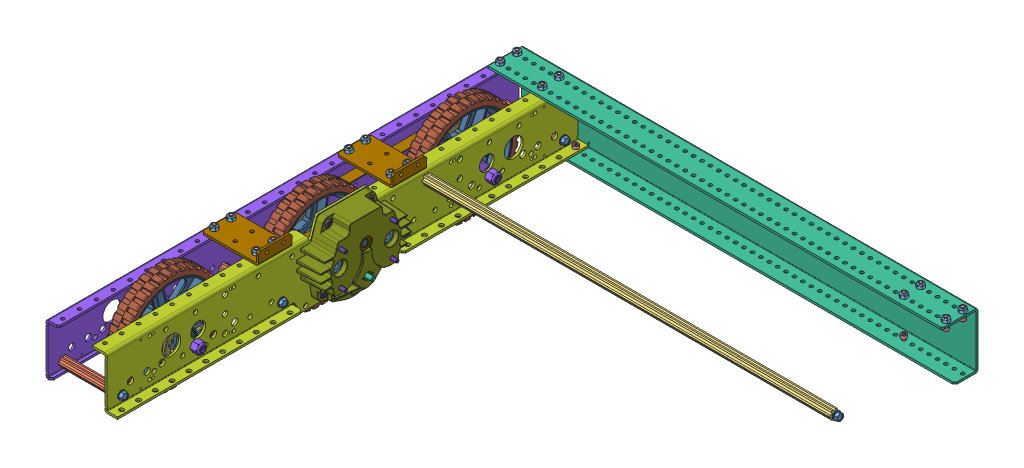
SolidWorks assembly AM14U3 Square Half, configuration Default. Lengths in mm.
Overall size (722.96 215.27 715.14).
150 component instances, 35 part files, 6 mates.
Components (placement in the parent):
- AM14U3 Square Frame Half-1: AM14U3 Square Frame Half [Default] at (326.068 37.2757 -291.2758) size (722.38 116.33 715.14)
  - ThreadRollingScrew_0.25-20x0.75_FHTS 0.25-20-G-0.75-C-1: ThreadRollingScrew_0.25-20x0.75_FHTS 0.25-20-G-0.75-C [Default] at (-600.075 -67.691 639.064) x (-1 0 0) z (0 0.924225 0.381849) size (24.64 12.19 12.19)
  - ThreadRollingScrew_0.25-20x0.75_FHTS 0.25-20-G-0.75-C-2: ThreadRollingScrew_0.25-20x0.75_FHTS 0.25-20-G-0.75-C [Default] at (-600.075 -67.691 -27.94) x (-1 0 0) z (0 0.924225 0.381849) size (24.64 12.19 12.19)
  - ThreadRollingScrew_0.25-20x0.75_FHTS 0.25-20-G-0.75-C-3: ThreadRollingScrew_0.25-20x0.75_FHTS 0.25-20-G-0.75-C [Default] at (-692.15 -67.691 -27.813) size (24.64 12.19 12.19)
  - ThreadRollingScrew_0.25-20x0.75_FHTS 0.25-20-G-0.75-C-4: ThreadRollingScrew_0.25-20x0.75_FHTS 0.25-20-G-0.75-C [Default] at (-603.25 -15.494 178.562) size (24.64 12.19 12.19)
  - ThreadRollingScrew_0.25-20x0.75_FHTS 0.25-20-G-0.75-C-5: ThreadRollingScrew_0.25-20x0.75_FHTS 0.25-20-G-0.75-C [Default] at (-692.15 -67.691 638.937) size (24.64 12.19 12.19)
  - ThreadRollingScrew_0.25-20x0.75_FHTS 0.25-20-G-0.75-C-6: ThreadRollingScrew_0.25-20x0.75_FHTS 0.25-20-G-0.75-C [Default] at (19.05 -15.494 178.562) x (-1 0 0) z (0 0.525103 -0.851039) size (24.64 12.19 12.19)
  - 500Churro_3.375-1: 500Churro_3.375 [Default] at (-603.25 -67.691 -27.813) x (0 -0.866025 0.5) z (-1 0 0) size (14.66 12.7 85.72)
  - 500Churro_3.375-2: 500Churro_3.375 [Default] at (-603.25 -67.691 638.937) x (0 -0.866025 0.5) z (-1 0 0) size (14.66 12.7 85.72)
  - 500Churro_24.25-1: 500Churro_24.25 [Default] at (15.875 -15.494 178.562) x (0 0 -1) z (-1 0 0) size (14.66 12.7 615.95)
  - Screw_SHCS_10-32x0.5_HX-SHCS 0.19-32x1.375x1-C-1: Screw_SHCS_10-32x0.5_HX-SHCS 0.19-32x1.375x1-C [Default] at (-679.45 -11.43 -11.938) x (0 1 0) z (-0.440454 0 0.897775) size (17.53 7.94 7.94)
  - Screw_SHCS_10-32x0.5_HX-SHCS 0.19-32x1.375x1-C-2: Screw_SHCS_10-32x0.5_HX-SHCS 0.19-32x1.375x1-C [Default] at (-679.45 -11.43 -37.338) x (0 1 0) z (-0.063425 0 0.997987) size (17.53 7.94 7.94)
  - Screw_SHCS_10-32x0.5_HX-SHCS 0.19-32x1.375x1-C-3: Screw_SHCS_10-32x0.5_HX-SHCS 0.19-32x1.375x1-C [Default] at (-615.95 -11.43 -37.338) x (0 1 0) z (0 0 1) size (17.53 7.94 7.94)
  - Screw_SHCS_10-32x0.5_HX-SHCS 0.19-32x1.375x1-C-4: Screw_SHCS_10-32x0.5_HX-SHCS 0.19-32x1.375x1-C [Default] at (-615.95 -11.43 -11.938) x (0 1 0) z (0 0 1) size (17.53 7.94 7.94)
  - Screw_SHCS_10-32x0.5_HX-SHCS 0.19-32x1.375x1-C-5: Screw_SHCS_10-32x0.5_HX-SHCS 0.19-32x1.375x1-C [Default] at (-590.55 -73.152 -37.338) x (0 -1 0) z (0 0 1) size (17.53 7.94 7.94)
  - Screw_SHCS_10-32x0.5_HX-SHCS 0.19-32x1.375x1-C-6: Screw_SHCS_10-32x0.5_HX-SHCS 0.19-32x1.375x1-C [Default] at (-6.35 -11.176 -37.338) x (0 1 0) z (0.222581 0 0.974914) size (17.53 7.94 7.94)
  - Screw_SHCS_10-32x0.5_HX-SHCS 0.19-32x1.375x1-C-7: Screw_SHCS_10-32x0.5_HX-SHCS 0.19-32x1.375x1-C [Default] at (-6.35 -11.176 -11.938) x (0 1 0) z (0.81526 0 0.579096) size (17.53 7.94 7.94)
  - Screw_SHCS_10-32x0.5_HX-SHCS 0.19-32x1.375x1-C-8: Screw_SHCS_10-32x0.5_HX-SHCS 0.19-32x1.375x1-C [Default] at (-69.85 -11.176 -37.338) x (0 1 0) z (0 0 1) size (17.53 7.94 7.94)
  - Screw_SHCS_10-32x0.5_HX-SHCS 0.19-32x1.375x1-C-9: Screw_SHCS_10-32x0.5_HX-SHCS 0.19-32x1.375x1-C [Default] at (-69.85 -11.176 -11.938) x (0 1 0) z (0.111454 0 0.99377) size (17.53 7.94 7.94)
  - Screw_SHCS_10-32x0.5_HX-SHCS 0.19-32x1.375x1-C-10: Screw_SHCS_10-32x0.5_HX-SHCS 0.19-32x1.375x1-C [Default] at (-95.25 -73.406 -37.338) x (0 -1 0) z (0.007214 0 0.999974) size (17.53 7.94 7.94)
  - 10-32 Nylock Nut-1: 10-32 Nylock Nut [Default] at (-679.45 0 -37.338) x (1 0 0) z (0 1 0) size (9.53 11 5.96)
  - 10-32 Nylock Nut-2: 10-32 Nylock Nut [Default] at (-679.45 0 -11.938) x (0.114693 0 0.993401) z (0 1 0) size (9.53 11 5.96)
  - 10-32 Nylock Nut-3: 10-32 Nylock Nut [Default] at (-615.95 0 -11.938) x (1 0 0) z (0 1 0) size (9.53 11 5.96)
  - 10-32 Nylock Nut-4: 10-32 Nylock Nut [Default] at (-615.95 0 -37.338) x (1 0 0) z (0 1 0) size (9.53 11 5.96)
  - 10-32 Nylock Nut-5: 10-32 Nylock Nut [Default] at (-69.85 0 -11.938) x (1 0 0) z (0 1 0) size (9.53 11 5.96)
  - 10-32 Nylock Nut-6: 10-32 Nylock Nut [Default] at (-69.85 0 -37.338) x (1 0 0) z (0 1 0) size (9.53 11 5.96)
  - 10-32 Nylock Nut-7: 10-32 Nylock Nut [Default] at (-6.35 0 -11.938) x (1 0 0) z (0 1 0) size (9.53 11 5.96)
  - 10-32 Nylock Nut-8: 10-32 Nylock Nut [Default] at (-6.35 0 -37.338) x (1 0 0) z (0 1 0) size (9.53 11 5.96)
  - 10-32 Nylock Nut-9: 10-32 Nylock Nut [Default] at (-95.25 -84.582 -37.338) x (1 0 0) z (0 -1 0) size (9.53 11 5.96)
  - 10-32 Nylock Nut-10: 10-32 Nylock Nut [Default] at (-590.55 -84.582 -37.338) x (1 0 0) z (0 -1 0) size (9.53 11 5.96)
  - Screw_SHCS_10-32x0.5_HX-SHCS 0.19-32x1.375x1-C-11: Screw_SHCS_10-32x0.5_HX-SHCS 0.19-32x1.375x1-C [Default] at (-679.45 -11.43 191.262) x (0 1 0) z (0 0 1) size (17.53 7.94 7.94)
  - Screw_SHCS_10-32x0.5_HX-SHCS 0.19-32x1.375x1-C-12: Screw_SHCS_10-32x0.5_HX-SHCS 0.19-32x1.375x1-C [Default] at (-679.45 -11.43 216.662) x (0 1 0) z (0 0 1) size (17.53 7.94 7.94)
  - Screw_SHCS_10-32x0.5_HX-SHCS 0.19-32x1.375x1-C-13: Screw_SHCS_10-32x0.5_HX-SHCS 0.19-32x1.375x1-C [Default] at (-615.95 -11.43 191.262) x (0 1 0) z (0 0 1) size (17.53 7.94 7.94)
  - Screw_SHCS_10-32x0.5_HX-SHCS 0.19-32x1.375x1-C-14: Screw_SHCS_10-32x0.5_HX-SHCS 0.19-32x1.375x1-C [Default] at (-615.95 -11.43 216.662) x (0 1 0) z (0 0 1) size (17.53 7.94 7.94)
  - Screw_SHCS_10-32x0.5_HX-SHCS 0.19-32x1.375x1-C-15: Screw_SHCS_10-32x0.5_HX-SHCS 0.19-32x1.375x1-C [Default] at (-615.95 -11.43 394.462) x (0 1 0) z (0 0 1) size (17.53 7.94 7.94)
  - Screw_SHCS_10-32x0.5_HX-SHCS 0.19-32x1.375x1-C-16: Screw_SHCS_10-32x0.5_HX-SHCS 0.19-32x1.375x1-C [Default] at (-615.95 -11.43 419.862) x (0 1 0) z (0 0 1) size (17.53 7.94 7.94)
  - Screw_SHCS_10-32x0.5_HX-SHCS 0.19-32x1.375x1-C-17: Screw_SHCS_10-32x0.5_HX-SHCS 0.19-32x1.375x1-C [Default] at (-679.45 -11.43 394.462) x (0 1 0) z (0 0 1) size (17.53 7.94 7.94)
  - Screw_SHCS_10-32x0.5_HX-SHCS 0.19-32x1.375x1-C-18: Screw_SHCS_10-32x0.5_HX-SHCS 0.19-32x1.375x1-C [Default] at (-679.45 -11.43 419.862) x (0 1 0) z (0 0 1) size (17.53 7.94 7.94)
  - 10-32 Nylock Nut-11: 10-32 Nylock Nut [Default] at (-679.45 -0.254 419.862) x (1 0 0) z (0 1 0) size (9.53 11 5.96)
  - 10-32 Nylock Nut-12: 10-32 Nylock Nut [Default] at (-679.45 -0.254 394.462) x (1 0 0) z (0 1 0) size (9.53 11 5.96)
  - 10-32 Nylock Nut-13: 10-32 Nylock Nut [Default] at (-615.95 -0.254 394.462) x (1 0 0) z (0 1 0) size (9.53 11 5.96)
  - 10-32 Nylock Nut-14: 10-32 Nylock Nut [Default] at (-615.95 -0.254 419.862) x (1 0 0) z (0 1 0) size (9.53 11 5.96)
  - 10-32 Nylock Nut-15: 10-32 Nylock Nut [Default] at (-679.45 -0.254 216.662) x (1 0 0) z (0 1 0) size (9.53 11 5.96)
  - 10-32 Nylock Nut-16: 10-32 Nylock Nut [Default] at (-679.45 -0.254 191.262) x (1 0 0) z (0 1 0) size (9.53 11 5.96)
  - 10-32 Nylock Nut-17: 10-32 Nylock Nut [Default] at (-615.95 -0.254 216.662) x (1 0 0) z (0 1 0) size (9.53 11 5.96)
  - 10-32 Nylock Nut-18: 10-32 Nylock Nut [Default] at (-615.95 -0.254 191.262) x (1 0 0) z (0 1 0) size (9.53 11 5.96)
  - AM14U3EndPlate_Square-1: AM14U3EndPlate_Square [Default] at (-787.4 -81.407 -53.975) x (1 0 0) z (0 -1 0) size (685.8 53.98 84.58)
  - AM14U3InnerPlate_Square-1: AM14U3InnerPlate_Square [Default] at (-603.25 -77.216 711.962) x (0 0 -1) z (0 -1 0) size (711.2 38.1 116.33)
  - AM14U3OuterPlate_Square-1: AM14U3OuterPlate_Square [Default] at (-667.7485 -27.0221 21.6115) x (0 0 1) z (0 -1 0) size (711.2 19.05 77.72)
  - Bracket_2x3-1: Bracket_2x3 [Default] at (-685.8 -3.429 445.262) size (85.72 19.05 50.8)
  - Bracket_2x3-2: Bracket_2x3 [Default] at (-685.8 -3.429 242.062) size (85.72 19.05 50.8)
  - 500Churro_3.375-3: 500Churro_3.375 [Default] at (-688.975 -66.929 397.637) x (0 0.428755 -0.903421) z (1 0 0) size (14.66 12.7 85.72)
  - 500Churro_3.375-4: 500Churro_3.375 [Default] at (-688.975 -66.929 213.487) x (0 0 -1) z (1 0 0) size (14.66 12.7 85.72)
  - ThreadRollingScrew_0.25-20x0.75_FHTS 0.25-20-G-0.75-C-7: ThreadRollingScrew_0.25-20x0.75_FHTS 0.25-20-G-0.75-C [Default] at (-600.075 -66.929 397.637) x (-1 0 0) z (0 0.924225 0.381849) size (24.64 12.19 12.19)
  - ThreadRollingScrew_0.25-20x0.75_FHTS 0.25-20-G-0.75-C-8: ThreadRollingScrew_0.25-20x0.75_FHTS 0.25-20-G-0.75-C [Default] at (-600.075 -66.929 213.487) x (-1 0 0) z (0 0.924225 0.381849) size (24.64 12.19 12.19)
  - ThreadRollingScrew_0.25-20x0.75_FHTS 0.25-20-G-0.75-C-9: ThreadRollingScrew_0.25-20x0.75_FHTS 0.25-20-G-0.75-C [Default] at (-692.15 -66.929 397.637) x (1 0 0) z (0 -0.467404 -0.884044) size (24.64 12.19 12.19)
  - ThreadRollingScrew_0.25-20x0.75_FHTS 0.25-20-G-0.75-C-10: ThreadRollingScrew_0.25-20x0.75_FHTS 0.25-20-G-0.75-C [Default] at (-692.15 -66.929 213.487) size (24.64 12.19 12.19)
- ToughboxMini-1: ToughboxMini [Default] at (-324.5487 -32.7384 105.387) x (0 0.001296 0.999999) z (-1 0 0) size (140.05 127.01 142.29)
  - TBMiniSmallHexShaft-1: TBMiniSmallHexShaft [Default] at (-129.7894 33.1737 -52.3959) x (-0.674239 -0.738513 0) z (-0.738513 0.674239 0) size (11 38.23 9.52)
  - LargeClusterGear_Hex_50t0.375-1: LargeClusterGear_Hex_50t0.375 [Default] at (-91.0349 50.9043 -67.5597) x (-0.674239 -0.738513 0) z (0 0 -1) size (65.97 66.04 10.34)
  - Bearing_FR6ZZ-1: Bearing_FR6ZZ [Default] at (-96.247 60.278 -52.5991) x (-0.893862 0.448342 0) z (0 0 1) size (24.69 24.69 7.16)
  - NylockNut_10-32-1: NylockNut_10-32 [Default] at (-129.8464 -8.0737 -56.3837) x (0.501678 0.865055 0) z (0 0 -1) size (9.53 11 5.96)
  - NylockNut_10-32-2: NylockNut_10-32 [Default] at (-59.2462 80.7349 -56.3837) x (0.999999 -0.001296 0) z (0 0 -1) size (9.53 11 5.96)
  - NylockNut_10-32-3: NylockNut_10-32 [Default] at (-122.7461 80.8172 -56.3837) x (0.500567 0.865698 0) z (0 0 -1) size (9.53 11 5.96)
  - NylockNut_10-32-4: NylockNut_10-32 [Default] at (-52.3764 -8.1741 -56.3837) x (-0.501678 -0.865055 0) z (0 0 -1) size (9.53 11 5.96)
  - Washer_5-16-1: Washer_5-16 [Default] at (-52.3162 38.3079 -77.7705) x (-0.418041 0.908428 0) z (0 0 -1) size (17.53 17.53 1.47)
  - Washer_5-16-2: Washer_5-16 [Default] at (-52.3162 38.3079 -76.2973) x (0.897267 -0.441488 0) z (0 0 -1) size (17.53 17.53 1.47)
  - Washer_5-16-3: Washer_5-16 [Default] at (-129.7861 38.4083 -77.7705) x (-0.990116 0.140253 0) z (0 0 1) size (17.53 17.53 1.47)
  - Washer_5-16-4: Washer_5-16 [Default] at (-129.7861 38.4083 -79.2437) x (-0.681761 0.731575 0) z (0 0 1) size (17.53 17.53 1.47)
  - CIMGear_14t8mm-1: CIMGear_14t8mm [Default] at (-52.3162 38.3079 -63.5973) x (-0.082762 0.996569 0) z (0 0 -1) size (20.03 20.32 12.7)
  - CIMGear_14t8mm-2: CIMGear_14t8mm [Default] at (-129.7861 38.4083 -63.5973) x (0.603285 0.797525 0) z (0 0 -1) size (20.03 20.32 12.7)
  - TBMiniHousing-1: TBMiniHousing [Default] at (-91.0876 10.1882 -86.3557) x (0.999999 -0.001296 0) z (0 0 1) size (139.9 118.55 41.62)
  - Screw_SHCS_10-32x0.625-1: Screw_SHCS_10-32x0.625 [Default] at (-52.2832 63.7078 -74.4685) x (-0.564778 -0.825243 0) z (-0.825243 0.564778 0) size (7.82 20.65 7.82)
  - Screw_SHCS_10-32x0.625-2: Screw_SHCS_10-32x0.625 [Default] at (-122.7461 80.8172 -42.5915) x (0.507484 -0.861661 0) z (-0.861661 -0.507484 0) size (7.82 20.65 7.82)
  - Screw_SHCS_10-32x0.625-3: Screw_SHCS_10-32x0.625 [Default] at (-52.3764 -8.1741 -42.5915) x (0.507484 -0.861661 0) z (-0.861661 -0.507484 0) size (7.82 20.65 7.82)
  - Screw_SHCS_10-32x0.625-4: Screw_SHCS_10-32x0.625 [Default] at (-129.8464 -8.0737 -42.5915) x (0.507484 -0.861661 0) z (-0.861661 -0.507484 0) size (7.82 20.65 7.82)
  - Screw_SHCS_10-32x0.625-5: Screw_SHCS_10-32x0.625 [Default] at (-59.2462 80.7349 -42.5915) x (0.740711 -0.671824 0) z (-0.671824 -0.740711 0) size (7.82 20.65 7.82)
  - Screw_SHCS_10-32x0.625-6: Screw_SHCS_10-32x0.625 [Default] at (-52.3491 12.9079 -74.4685) x (-0.564778 -0.825243 0) z (-0.825243 0.564778 0) size (7.82 20.65 7.82)
  - Screw_SHCS_10-32x0.625-7: Screw_SHCS_10-32x0.625 [Default] at (-129.7532 63.8083 -74.4685) x (-0.966277 -0.257503 0) z (-0.257503 0.966277 0) size (7.82 20.65 7.82)
  - Screw_SHCS_10-32x0.625-8: Screw_SHCS_10-32x0.625 [Default] at (-129.819 13.0083 -74.4685) x (-0.99652 0.083357 0) z (0.083357 0.99652 0) size (7.82 20.65 7.82)
  - Bearing_R6ZZ-1: Bearing_R6ZZ [Default] at (-91.0349 50.9043 -84.8317) x (0.958138 -0.286306 0) z (0 0 1) size (22.23 22.23 7.11)
  - Bearing_R6ZZ-2: Bearing_R6ZZ [Default] at (-91.0876 10.1882 -84.8317) x (-0.661529 0.74992 0) z (0 0 1) size (22.23 22.23 7.11)
  - RetainingClip-1: RetainingClip [Default] at (-129.7861 38.4083 -63.5973) x (0 0 1) z (-1 0 0) size (1.12 14.83 14.83)
  - RetainingClip-2: RetainingClip [Default] at (-52.3162 38.3079 -63.5973) x (0 0 1) z (-1 0 0) size (1.12 14.83 14.83)
  - ExternalKlipring-1: ExternalKlipring [Default] at (-91.0876 10.1882 -64.4355) x (0.996411 -0.084651 0) z (0 0 1) size (19.07 20.96 1.27)
  - Bearing_Hex_FR8ZZ-1: Bearing_Hex_FR8ZZ [Default] at (-91.0876 10.1882 -44.6717) x (0.73373 0.679441 0) z (0 0 -1) size (31.12 31.12 7.93)
  - SmallClusterGear_Hex_16t0.375-1: SmallClusterGear_Hex_16t0.375 [Default] at (-91.0349 50.9043 -67.5597) x (0 0 1) z (0.302452 -0.953165 0) size (15.19 22.57 22.57)
  - LargeOutputGear_Hex_48t0.5-1: LargeOutputGear_Hex_48t0.5 [Default] at (-91.0876 10.1882 -63.1655) x (0 0 1) z (-0.955278 0.295708 0) size (10.21 63.42 63.42)
  - TBMiniHexOutputShaft-1: TBMiniHexOutputShaft [Default] at (-51.6549 23.9851 -52.3197) x (0.73373 0.679441 0) z (0.679441 -0.73373 0) size (14.66 142.29 12.7)
- Bearing_Hex_FR8ZZ-1: Bearing_Hex_FR8ZZ [Default] at (-369.3104 -22.6683 14.2862) x (0 -0.974861 0.222813) z (1 0 0) size (31.12 31.12 7.93)
- hex finished bolt_ai_HFBOLT 0.375-16x2.5x1-C-1: hex finished bolt_ai_HFBOLT 0.375-16x2.5x1-C [Default] at (-372.2542 -20.8903 236.8339) size (69.67 16.48 14.27)
- hex finished bolt_ai_HFBOLT 0.375-16x2.5x1-C-2: hex finished bolt_ai_HFBOLT 0.375-16x2.5x1-C [Default] at (-372.2542 -20.8903 -208.2615) size (69.67 16.48 14.27)
- NylockNut_0.375-16_91831A127-1: NylockNut_0.375-16_91831A127 [Default] at (-274.007 -20.8903 236.8339) x (0 -1 0) z (0 0 1) size (14.29 12 16.5)
- NylockNut_0.375-16_91831A127-2: NylockNut_0.375-16_91831A127 [Default] at (-274.007 -20.8903 -208.2615) x (0 -1 0) z (0 0 1) size (14.29 12 16.5)
- Belt_15mm_Square-1: Belt_15mm_Square [Default] at (-289.0679 -20.8903 236.8339) x (0 -0.007989 -0.999968) z (-1 0 0) size (291.74 69.19 15)
- Belt_15mm_Square-2: Belt_15mm_Square [Default] at (-335.856 -20.8903 -208.2615) x (0 -0.007989 0.999968) z (-1 0 0) size (291.74 69.19 15)
- 6 HiGrip with hub and double pulley-1: 6 HiGrip with hub and double pulley [Default] at (-288.8079 95.5145 -82.9912) x (-1 0 0) z (0 -0.348575 0.937281) size (80.63 152.4 152.4)
  - 6 HiGrip Wheel Assembly Rev II-1: 6 HiGrip Wheel Assembly Rev II [Default] at (83.7987 67.439 110.9939) size (34.93 152.4 152.4)
    - 6 wheel Rev 4-1: 6 wheel Rev 4 [Default] at (-52.6446 9.4231 21.378) size (34.93 132.08 132.08)
    - 6 wheel tread II-1: 6 wheel tread II [Default] at (-65.3446 9.4231 21.378) x (0 0 -1) z (1 0 0) size (152.4 152.4 25.58)
  - HalfPulley_42t5mm-1: HalfPulley_42t5mm [Default] at (47.6006 76.862 132.3719) x (1 0 0) z (0 -0.5 0.866025) size (13 74.23 74.23)
  - HalfPulley_42t5mm-2: HalfPulley_42t5mm [Default] at (64.263 76.862 132.3719) x (-1 0 0) z (0 -0.499927 0.866067) size (13 74.23 74.23)
  - Washer_5-16-1: Washer_5-16 [Default] at (63.247 76.8605 108.5602) x (0 -0.812665 -0.582732) z (1 0 0) size (17.53 17.53 1.47)
  - Washer_5-16-2: Washer_5-16 [Default] at (63.247 97.4833 120.4656) x (0 0.998209 0.059825) z (1 0 0) size (17.53 17.53 1.47)
  - Washer_5-16-3: Washer_5-16 [Default] at (63.247 56.2398 144.2799) x (0 -0.026074 -0.99966) z (1 0 0) size (17.53 17.53 1.47)
  - Washer_5-16-4: Washer_5-16 [Default] at (63.247 76.8625 156.1852) x (0 -0.766208 -0.642593) z (1 0 0) size (17.53 17.53 1.47)
  - Washer_5-16-5: Washer_5-16 [Default] at (63.247 97.4843 144.2781) x (0 -0.833184 -0.552996) z (1 0 0) size (17.53 17.53 1.47)
  - Washer_5-16-6: Washer_5-16 [Default] at (63.247 56.2388 120.4674) x (0 -0.998572 0.053424) z (1 0 0) size (17.53 17.53 1.47)
  - HalfPulley_42t5mm-3: HalfPulley_42t5mm [Default] at (-1.9548 76.8628 132.3714) x (1 0 0) z (0 -1 -0.000063) size (13 74.23 74.23)
  - HalfPulley_42t5mm-4: HalfPulley_42t5mm [Default] at (14.7076 76.8628 132.3714) x (-1 0 0) z (0 -1 0.000021) size (13 74.23 74.23)
  - HexHub_500EX-1: HexHub_500EX [Default] at (-8.3048 76.862 132.3719) x (0 -0.866025 -0.5) z (0 -0.5 0.866025) size (55.37 25.4 51.33)
  - Washer_5-16-7: Washer_5-16 [Default] at (-5.2568 97.4843 120.4656) x (0 0.577286 0.816542) z (-1 0 0) size (17.53 17.53 1.47)
  - Washer_5-16-8: Washer_5-16 [Default] at (-5.2568 76.862 108.5594) x (0 0.877244 0.480045) z (-1 0 0) size (17.53 17.53 1.47)
  - Washer_5-16-9: Washer_5-16 [Default] at (-5.2568 56.2398 120.4656) x (0 -0.894136 -0.447796) z (-1 0 0) size (17.53 17.53 1.47)
  - Washer_5-16-10: Washer_5-16 [Default] at (-5.2568 97.4843 144.2781) x (0 -0.559623 -0.828747) z (-1 0 0) size (17.53 17.53 1.47)
  - Washer_5-16-11: Washer_5-16 [Default] at (-5.2568 56.2398 144.2781) x (0 -0.82184 -0.569719) z (-1 0 0) size (17.53 17.53 1.47)
  - Washer_5-16-12: Washer_5-16 [Default] at (-5.2568 76.862 156.1844) x (0 -0.981812 0.189856) z (-1 0 0) size (17.53 17.53 1.47)
  - Spacer_Hex_0.57x0.5-1: Spacer_Hex_0.57x0.5 [Default] at (57.8495 76.862 132.3719) x (0 -0.866025 -0.5) z (0 -0.5 0.866025) size (28.55 14.48 28.55)
- 6 HiGrip with bearings, pulleys and spacers_2-1: 6 HiGrip with bearings, pulleys and spacers_2 [Default] at (-287.4242 44.9655 -70.0838) x (-1 0 0) z (0 -0.825353 -0.564617) size (85.56 152.4 152.4)
  - 6 HiGrip Wheel Assembly Rev II-1: 6 HiGrip Wheel Assembly Rev II [Default] at (83.7987 67.439 110.9939) size (34.93 152.4 152.4)
    - 6 wheel Rev 4-1: 6 wheel Rev 4 [Default] at (-52.6446 9.4231 21.378) size (34.93 132.08 132.08)
    - 6 wheel tread II-1: 6 wheel tread II [Default] at (-65.3446 9.4231 21.378) x (0 0 -1) z (1 0 0) size (152.4 152.4 25.58)
  - HalfPulley_42t5mm-1: HalfPulley_42t5mm [Default] at (47.6006 76.862 132.3719) x (1 0 0) z (0 -0.5 0.866025) size (13 74.23 74.23)
  - HalfPulley_42t5mm-2: HalfPulley_42t5mm [Default] at (64.263 76.862 132.3719) x (-1 0 0) z (0 -0.499927 0.866067) size (13 74.23 74.23)
  - Bearing_1614ZZ-1: Bearing_1614ZZ [Default] at (62.612 76.862 132.3719) x (0 -0.157148 -0.987575) z (-1 0 0) size (28.58 28.58 9.53)
  - Bearing_1614ZZ-2: Bearing_1614ZZ [Default] at (15.2791 76.862 132.3719) x (0 0 -1) z (1 0 0) size (28.58 28.58 9.53)
  - Washer_5-16-1: Washer_5-16 [Default] at (63.247 76.8605 108.5602) x (0 0.946124 0.323805) z (1 0 0) size (17.53 17.53 1.47)
  - Washer_5-16-2: Washer_5-16 [Default] at (63.247 97.4833 120.4656) x (0 0.770474 -0.637472) z (1 0 0) size (17.53 17.53 1.47)
  - Washer_5-16-3: Washer_5-16 [Default] at (63.247 56.2398 144.2799) x (0 0 -1) z (1 0 0) size (17.53 17.53 1.47)
  - Washer_5-16-4: Washer_5-16 [Default] at (63.247 76.8625 156.1852) x (0 -0.95788 -0.287168) z (1 0 0) size (17.53 17.53 1.47)
  - Washer_5-16-5: Washer_5-16 [Default] at (63.247 97.4843 144.2781) x (0 -0.653102 0.75727) z (1 0 0) size (17.53 17.53 1.47)
  - Washer_5-16-6: Washer_5-16 [Default] at (63.247 56.2388 120.4674) x (0 -0.977348 -0.211637) z (1 0 0) size (17.53 17.53 1.47)
  - Spacer_0.28x0.382-1: Spacer_0.28x0.382 [Default] at (74.4865 76.862 132.3719) x (0 -0.35357 0.935408) z (-1 0 0) size (13.16 13.16 7.11)
  - Spacer_0.85x0.38-1: Spacer_0.85x0.38 [Default] at (-11.0734 76.862 132.3719) x (0 0 -1) z (1 0 0) size (19.05 19.05 21.59)
- 6 HiGrip with bearings, pulleys and spacers_2-2: 6 HiGrip with bearings, pulleys and spacers_2 [Default] at (-352.4997 11.0539 87.1353) x (1 0 0) z (0 -0.671558 0.740952) size (85.56 152.4 152.4)
  - 6 HiGrip Wheel Assembly Rev II-1: 6 HiGrip Wheel Assembly Rev II [Default] at (83.7987 67.439 110.9939) size (34.93 152.4 152.4)
    - 6 wheel Rev 4-1: 6 wheel Rev 4 [Default] at (-52.6446 9.4231 21.378) size (34.93 132.08 132.08)
    - 6 wheel tread II-1: 6 wheel tread II [Default] at (-65.3446 9.4231 21.378) x (0 0 -1) z (1 0 0) size (152.4 152.4 25.58)
  - HalfPulley_42t5mm-1: HalfPulley_42t5mm [Default] at (47.6006 76.862 132.3719) x (1 0 0) z (0 -0.5 0.866025) size (13 74.23 74.23)
  - HalfPulley_42t5mm-2: HalfPulley_42t5mm [Default] at (64.263 76.862 132.3719) x (-1 0 0) z (0 -0.499927 0.866067) size (13 74.23 74.23)
  - Bearing_1614ZZ-1: Bearing_1614ZZ [Default] at (62.612 76.862 132.3719) x (0 -0.157148 -0.987575) z (-1 0 0) size (28.58 28.58 9.53)
  - Bearing_1614ZZ-2: Bearing_1614ZZ [Default] at (15.2791 76.862 132.3719) x (0 0 -1) z (1 0 0) size (28.58 28.58 9.53)
  - Washer_5-16-1: Washer_5-16 [Default] at (63.247 76.8605 108.5602) x (0 0.946124 0.323805) z (1 0 0) size (17.53 17.53 1.47)
  - Washer_5-16-2: Washer_5-16 [Default] at (63.247 97.4833 120.4656) x (0 0.770474 -0.637472) z (1 0 0) size (17.53 17.53 1.47)
  - Washer_5-16-3: Washer_5-16 [Default] at (63.247 56.2398 144.2799) x (0 0 -1) z (1 0 0) size (17.53 17.53 1.47)
  - Washer_5-16-4: Washer_5-16 [Default] at (63.247 76.8625 156.1852) x (0 -0.95788 -0.287168) z (1 0 0) size (17.53 17.53 1.47)
  - Washer_5-16-5: Washer_5-16 [Default] at (63.247 97.4843 144.2781) x (0 -0.653102 0.75727) z (1 0 0) size (17.53 17.53 1.47)
  - Washer_5-16-6: Washer_5-16 [Default] at (63.247 56.2388 120.4674) x (0 -0.977348 -0.211637) z (1 0 0) size (17.53 17.53 1.47)
  - Spacer_0.28x0.382-1: Spacer_0.28x0.382 [Default] at (74.4865 76.862 132.3719) x (0 -0.35357 0.935408) z (-1 0 0) size (13.16 13.16 7.11)
  - Spacer_0.85x0.38-1: Spacer_0.85x0.38 [Default] at (-11.0734 76.862 132.3719) x (0 0 -1) z (1 0 0) size (19.05 19.05 21.59)
Mates (geometry in assembly coordinates):
- Concentric2: concentric anti-aligned: cylinder of hex finished bolt_ai_HFBOLT 0.375-16x2.5x1-C-2 through (-372.2542 -20.8903 -208.2615) axis (-1 0 0) radius 4.7625; cylinder of 6 HiGrip with bearings, pulleys and spacers_2-1/Spacer_0.85x0.38-1 through (-297.9408 -20.8903 -208.2615) axis (1 0 0) radius 4.826
- Coincident1: coincident aligned: axis of Bearing_Hex_FR8ZZ-1 through (-360.7194 -22.6683 14.2862) axis (-1 0 0); axis of 6 HiGrip with hub and double pulley-1/Spacer_Hex_0.57x0.5-1 through (-352.806 -22.6683 14.2862) axis (-1 0 0)
- Width1: width anti-aligned: plane of 6 HiGrip with hub and double pulley-1/HalfPulley_42t5mm-2 through (-355.6109 9.3414 8.875) normal (-1 0 0); plane of 6 HiGrip with hub and double pulley-1/HalfPulley_42t5mm-3 through (-284.3131 -33.9831 44.714) normal (1 0 0); plane of Belt_15mm_Square-1 through (-289.0679 -20.8903 236.8339) normal (1 0 0); plane of Belt_15mm_Square-2 through (-350.856 -20.8903 -208.2615) normal (-1 0 0)
- Concentric3: concentric aligned: cylinder of hex finished bolt_ai_HFBOLT 0.375-16x2.5x1-C-1 through (-372.2542 -20.8903 236.8339) axis (-1 0 0) radius 4.7625; cylinder of 6 HiGrip with bearings, pulleys and spacers_2-2/Spacer_0.85x0.38-1 through (-341.9831 -20.8903 236.8339) axis (-1 0 0) radius 4.826
- Width2: width anti-aligned: plane of 6 HiGrip with bearings, pulleys and spacers_2-1/HalfPulley_42t5mm-2 through (-354.2272 -23.3699 -175.8924) normal (-1 0 0); plane of 6 HiGrip with bearings, pulleys and spacers_2-1/HalfPulley_42t5mm-1 through (-332.4848 -18.4134 -240.6308) normal (1 0 0); plane of Belt_15mm_Square-2 through (-335.856 -20.8903 -208.2615) normal (1 0 0); plane of Belt_15mm_Square-2 through (-350.856 -20.8903 -208.2615) normal (-1 0 0)
- Width3: width anti-aligned: plane of 6 HiGrip with bearings, pulleys and spacers_2-2/HalfPulley_42t5mm-2 through (-285.6967 -30.8238 205.9271) normal (1 0 0); plane of 6 HiGrip with bearings, pulleys and spacers_2-2/HalfPulley_42t5mm-1 through (-307.4391 -10.9595 267.7415) normal (-1 0 0); plane of Belt_15mm_Square-1 through (-304.0679 -20.8903 236.8339) normal (-1 0 0); plane of Belt_15mm_Square-1 through (-289.0679 -20.8903 236.8339) normal (1 0 0)
